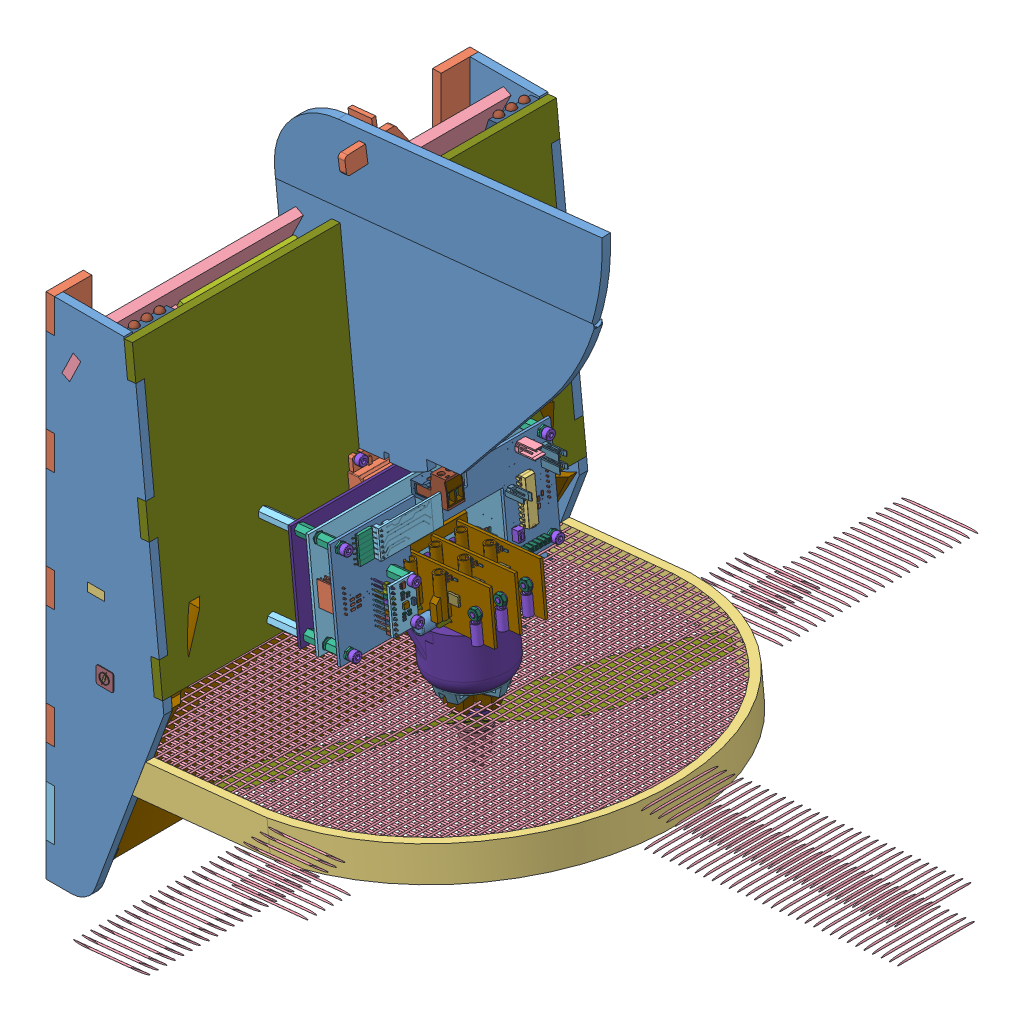
SolidWorks assembly AssTotale, configuration Défaut. Lengths in mm. (continued)
Components (placement in the parent): (continued)
- AssStructSimu-1: AssStructSimu [Défaut] at (-75.9431 -10.8604 24.5323) size (253.25 324.59 251.6) (continued)
  - AssCarte-1: AssCarte [Défaut] at (-42.8534 32.2132 302.028) x (-0.101852 0.9948 0) z (0.9948 0.101852 0) size (67.15 130.57 98.45) (continued)
    - carte_onduleur_v4-1: carte_onduleur_v4 [Défaut] at (-25.7639 0.8332 112.9379) size (66.52 130.57 82.34) (continued)
      - CARTE_CMD-1: CARTE_CMD [Défaut] at (25 57.2 0.803) size (60.1 130 26.71) (continued)
        - Open CASCADE STEP translator 6.8 1.20.1-1: Open CASCADE STEP translator 6.8 1.20.1 [Défaut] at origin size (60.1 130 26.71) (continued)
          - Body_1_4-1: Body_1_4 [Défaut] at (-55 5 12) size (60.1 130 26.71) (continued)
            - 175-1: 175 [Défaut] at (10 -21.7 0.803) x (0 -1 0) z (0 0 1) size (15 25.4 12.78) (continued)
              - =_[0_1_1_72]-1: =_[0_1_1_72] [Défaut] at origin size (15 25.4 12.78) (continued)
                - 173-1: 173 [Défaut] at (-1.4 -1 12) x (-1 0 0) z (0 1 0) size (15 12.78 25.4) (continued)
                  - RESC-0603_5-3: RESC-0603_5 [Défaut] at (-6.85 0 17.55) x (1 0 0) z (0 1 0) size (1.7 0.9 0.55) (continued)
                    - 152-1: 152 [Défaut] at origin (continued)
                      - =_[0_1_1_112]-1: =_[0_1_1_112] [Défaut] at origin
                      - =_[0_1_1_113]-1: =_[0_1_1_113] [Défaut] at origin
                      - =_[0_1_1_114]-1: =_[0_1_1_114] [Défaut] at origin
                      - =_[0_1_1_115]-1: =_[0_1_1_115] [Défaut] at origin
                  - RESC-0603_5-4: RESC-0603_5 [Défaut] at (-6.85 0 16.05) x (1 0 0) z (0 1 0) size (1.7 0.9 0.55)
                    - 143-1: 143 [Défaut] at origin size (1.7 0.9 0.55)
                      - =_[0_1_1_103]-1: =_[0_1_1_103] [Défaut] at origin size (0.4 0.9 0.53)
                      - =_[0_1_1_105]-1: =_[0_1_1_105] [Défaut] at origin size (0.4 0.9 0.53)
                      - =_[0_1_1_106]-1: =_[0_1_1_106] [Défaut] at origin size (1.64 0.9 0.52)
                    - 152-1: 152 [Défaut] at origin
                      - =_[0_1_1_107]-1: =_[0_1_1_107] [Défaut] at origin
                      - =_[0_1_1_109]-1: =_[0_1_1_109] [Défaut] at origin
                      - =_[0_1_1_110]-1: =_[0_1_1_110] [Défaut] at origin
                      - =_[0_1_1_111]-1: =_[0_1_1_111] [Défaut] at origin
                      - =_[0_1_1_112]-1: =_[0_1_1_112] [Défaut] at origin
                      - =_[0_1_1_113]-1: =_[0_1_1_113] [Défaut] at origin
                      - =_[0_1_1_114]-1: =_[0_1_1_114] [Défaut] at origin
                      - =_[0_1_1_115]-1: =_[0_1_1_115] [Défaut] at origin
                  - RESC-0603_5-5: RESC-0603_5 [Défaut] at (-6.85 0 5.95) x (1 0 0) z (0 1 0) size (1.7 0.9 0.55)
                    - 143-1: 143 [Défaut] at origin size (1.7 0.9 0.55)
                      - =_[0_1_1_103]-1: =_[0_1_1_103] [Défaut] at origin size (0.4 0.9 0.53)
                      - =_[0_1_1_105]-1: =_[0_1_1_105] [Défaut] at origin size (0.4 0.9 0.53)
                      - =_[0_1_1_106]-1: =_[0_1_1_106] [Défaut] at origin size (1.64 0.9 0.52)
                    - 152-1: 152 [Défaut] at origin
                      - =_[0_1_1_107]-1: =_[0_1_1_107] [Défaut] at origin
                      - =_[0_1_1_109]-1: =_[0_1_1_109] [Défaut] at origin
                      - =_[0_1_1_110]-1: =_[0_1_1_110] [Défaut] at origin
                      - =_[0_1_1_111]-1: =_[0_1_1_111] [Défaut] at origin
                      - =_[0_1_1_112]-1: =_[0_1_1_112] [Défaut] at origin
                      - =_[0_1_1_113]-1: =_[0_1_1_113] [Défaut] at origin
                      - =_[0_1_1_114]-1: =_[0_1_1_114] [Défaut] at origin
                      - =_[0_1_1_115]-1: =_[0_1_1_115] [Défaut] at origin
                  - CAPC-0603-T0.9-BN_5-1: CAPC-0603-T0.9-BN_5 [Défaut] at (-9.85 0 8.95) x (1 0 0) z (0 1 0) size (1.7 0.9 0.9)
                    - =_[0_1_1_117]-1: =_[0_1_1_117] [Défaut] at origin size (1.7 0.9 0.9)
                    - 167-1: 167 [Défaut] at origin
                      - =_[0_1_1_118]-1: =_[0_1_1_118] [Défaut] at origin
                      - =_[0_1_1_120]-1: =_[0_1_1_120] [Défaut] at origin
                      - =_[0_1_1_121]-1: =_[0_1_1_121] [Défaut] at origin
                      - =_[0_1_1_122]-1: =_[0_1_1_122] [Défaut] at origin
                      - =_[0_1_1_123]-1: =_[0_1_1_123] [Défaut] at origin
                      - =_[0_1_1_124]-1: =_[0_1_1_124] [Défaut] at origin
                      - =_[0_1_1_125]-1: =_[0_1_1_125] [Défaut] at origin
                      - =_[0_1_1_126]-1: =_[0_1_1_126] [Défaut] at origin
                  - CAPC-0603-T0.9-BN_5-2: CAPC-0603-T0.9-BN_5 [Défaut] at (-6.85 0 8.95) x (1 0 0) z (0 1 0) size (1.7 0.9 0.9)
                    - =_[0_1_1_117]-1: =_[0_1_1_117] [Défaut] at origin size (1.7 0.9 0.9)
                    - 167-1: 167 [Défaut] at origin
                      - =_[0_1_1_118]-1: =_[0_1_1_118] [Défaut] at origin
                      - =_[0_1_1_120]-1: =_[0_1_1_120] [Défaut] at origin
                      - =_[0_1_1_121]-1: =_[0_1_1_121] [Défaut] at origin
                      - =_[0_1_1_122]-1: =_[0_1_1_122] [Défaut] at origin
                      - =_[0_1_1_123]-1: =_[0_1_1_123] [Défaut] at origin
                      - =_[0_1_1_124]-1: =_[0_1_1_124] [Défaut] at origin
                      - =_[0_1_1_125]-1: =_[0_1_1_125] [Défaut] at origin
                      - =_[0_1_1_126]-1: =_[0_1_1_126] [Défaut] at origin
                  - CAPC-0603-T0.9-BN_5-3: CAPC-0603-T0.9-BN_5 [Défaut] at (-6.85 0 19.05) x (1 0 0) z (0 1 0) size (1.7 0.9 0.9)
                    - =_[0_1_1_117]-1: =_[0_1_1_117] [Défaut] at origin size (1.7 0.9 0.9)
                    - 167-1: 167 [Défaut] at origin
                      - =_[0_1_1_118]-1: =_[0_1_1_118] [Défaut] at origin
                      - =_[0_1_1_120]-1: =_[0_1_1_120] [Défaut] at origin
                      - =_[0_1_1_121]-1: =_[0_1_1_121] [Défaut] at origin
                      - =_[0_1_1_122]-1: =_[0_1_1_122] [Défaut] at origin
                      - =_[0_1_1_123]-1: =_[0_1_1_123] [Défaut] at origin
                      - =_[0_1_1_124]-1: =_[0_1_1_124] [Défaut] at origin
                      - =_[0_1_1_125]-1: =_[0_1_1_125] [Défaut] at origin
                      - =_[0_1_1_126]-1: =_[0_1_1_126] [Défaut] at origin
                  - CAPC-0603-T0.9-BN_5-4: CAPC-0603-T0.9-BN_5 [Défaut] at (-9.85 0 7.45) x (1 0 0) z (0 1 0) size (1.7 0.9 0.9)
                    - =_[0_1_1_117]-1: =_[0_1_1_117] [Défaut] at origin size (1.7 0.9 0.9)
                    - 167-1: 167 [Défaut] at origin
                      - =_[0_1_1_118]-1: =_[0_1_1_118] [Défaut] at origin
                      - =_[0_1_1_120]-1: =_[0_1_1_120] [Défaut] at origin
                      - =_[0_1_1_121]-1: =_[0_1_1_121] [Défaut] at origin
                      - =_[0_1_1_122]-1: =_[0_1_1_122] [Défaut] at origin
                      - =_[0_1_1_123]-1: =_[0_1_1_123] [Défaut] at origin
                      - =_[0_1_1_124]-1: =_[0_1_1_124] [Défaut] at origin
                      - =_[0_1_1_125]-1: =_[0_1_1_125] [Défaut] at origin
                      - =_[0_1_1_126]-1: =_[0_1_1_126] [Défaut] at origin
                  - CAPC-0603-T0.9-BN_5-5: CAPC-0603-T0.9-BN_5 [Défaut] at (-9.85 0 17.55) x (1 0 0) z (0 1 0) size (1.7 0.9 0.9)
                    - =_[0_1_1_117]-1: =_[0_1_1_117] [Défaut] at origin size (1.7 0.9 0.9)
                    - 167-1: 167 [Défaut] at origin
                      - =_[0_1_1_118]-1: =_[0_1_1_118] [Défaut] at origin
                      - =_[0_1_1_120]-1: =_[0_1_1_120] [Défaut] at origin
                      - =_[0_1_1_121]-1: =_[0_1_1_121] [Défaut] at origin
                      - =_[0_1_1_122]-1: =_[0_1_1_122] [Défaut] at origin
                      - =_[0_1_1_123]-1: =_[0_1_1_123] [Défaut] at origin
                      - =_[0_1_1_124]-1: =_[0_1_1_124] [Défaut] at origin
                      - =_[0_1_1_125]-1: =_[0_1_1_125] [Défaut] at origin
                      - =_[0_1_1_126]-1: =_[0_1_1_126] [Défaut] at origin
            - 177-1: 177 [Défaut] at (52.1 -16.5 -0.803) x (1 0 0) z (0 0 -1) size (2.34 1.04 0.5)
              - =_[0_1_1_30]-1: =_[0_1_1_30] [Défaut] at origin size (2.34 1.04 0.5)
                - 32_2-1: 32_2 [Défaut] at origin size (2.29 1.04 0.43)
                - 33_2-1: 33_2 [Défaut] at (0.3048 0 0) x (-1 0 0) z (0 0 1) size (0.51 1.02 0.5)
                - 34-1: 34 [Défaut] at origin size (0.51 1.02 0.5)
            - 179-1: 179 [Défaut] at (22.5336 -121.5 -0.803) x (-1 0 0) z (0 0 -1) size (2.34 1.04 0.5)
              - =_[0_1_1_30]-1: =_[0_1_1_30] [Défaut] at origin size (2.34 1.04 0.5)
                - 32_2-1: 32_2 [Défaut] at origin size (2.29 1.04 0.43)
                - 33_2-1: 33_2 [Défaut] at (0.3048 0 0) x (-1 0 0) z (0 0 1) size (0.51 1.02 0.5)
                - 34-1: 34 [Défaut] at origin size (0.51 1.02 0.5)
            - 181-1: 181 [Défaut] at (48.6 -127 -0.803) x (-1 0 0) z (0 0 -1) size (2.34 1.04 0.5)
              - =_[0_1_1_30]-1: =_[0_1_1_30] [Défaut] at origin size (2.34 1.04 0.5)
                - 32_2-1: 32_2 [Défaut] at origin size (2.29 1.04 0.43)
                - 33_2-1: 33_2 [Défaut] at (0.3048 0 0) x (-1 0 0) z (0 0 1) size (0.51 1.02 0.5)
                - 34-1: 34 [Défaut] at origin size (0.51 1.02 0.5)
            - 183-1: 183 [Défaut] at (26.0189 -121.5 0.803) size (2.34 1.04 0.5)
              - =_[0_1_1_30]-1: =_[0_1_1_30] [Défaut] at origin size (2.34 1.04 0.5)
                - 32_2-1: 32_2 [Défaut] at origin size (2.29 1.04 0.43)
                - 33_2-1: 33_2 [Défaut] at (0.3048 0 0) x (-1 0 0) z (0 0 1) size (0.51 1.02 0.5)
                - 34-1: 34 [Défaut] at origin size (0.51 1.02 0.5)
            - 185-1: 185 [Défaut] at (30.3664 -19 -0.803) x (1 0 0) z (0 0 -1) size (2.34 1.04 0.5)
              - =_[0_1_1_30]-1: =_[0_1_1_30] [Défaut] at origin size (2.34 1.04 0.5)
                - 32_2-1: 32_2 [Défaut] at origin size (2.29 1.04 0.43)
                - 33_2-1: 33_2 [Défaut] at (0.3048 0 0) x (-1 0 0) z (0 0 1) size (0.51 1.02 0.5)
                - 34-1: 34 [Défaut] at origin size (0.51 1.02 0.5)
            - 187-1: 187 [Défaut] at (51.7 -114.3 -0.803) x (0 1 0) z (0 0 -1) size (2.34 1.04 0.5)
              - =_[0_1_1_30]-1: =_[0_1_1_30] [Défaut] at origin size (2.34 1.04 0.5)
                - 32_2-1: 32_2 [Défaut] at origin size (2.29 1.04 0.43)
                - 33_2-1: 33_2 [Défaut] at (0.3048 0 0) x (-1 0 0) z (0 0 1) size (0.51 1.02 0.5)
                - 34-1: 34 [Défaut] at origin size (0.51 1.02 0.5)
            - 189-1: 189 [Défaut] at (50 -114.3 -0.803) x (0 1 0) z (0 0 -1) size (2.34 1.04 0.5)
              - =_[0_1_1_30]-1: =_[0_1_1_30] [Défaut] at origin size (2.34 1.04 0.5)
                - 32_2-1: 32_2 [Défaut] at origin size (2.29 1.04 0.43)
                - 33_2-1: 33_2 [Défaut] at (0.3048 0 0) x (-1 0 0) z (0 0 1) size (0.51 1.02 0.5)
                - 34-1: 34 [Défaut] at origin size (0.51 1.02 0.5)
            - 192-1: 192 [Défaut] at (37.94 -103.3308 0.803) x (-1 0 0) z (0 0 1) size (5.08 5 14.3)
              - =_[0_1_1_135]-1: =_[0_1_1_135] [Défaut] at origin size (5.08 5 14.3)
                - 190-1: 190 [Défaut] at (1.2 0 11) size (5.08 5 14.3)
            - 194-1: 194 [Défaut] at (32.7796 -102.6 -0.803) x (-1 0 0) z (0 0 -1) size (2.54 1.98 0.64)
              - =_[0_1_1_46]-1: =_[0_1_1_46] [Défaut] at origin size (2.54 1.98 0.64)
                - 52-1: 52 [Défaut] at origin size (2.54 1.14 0.58)
                - 53-1: 53 [Défaut] x (0 -1 0) z (0 0 1) size (0.43 0.51 0.38)
                - 54-1: 54 [Défaut] at (1.8796 1.8796 0) x (0 -1 0) z (0 0 1) size (0.43 0.51 0.38)
                - 55-1: 55 [Défaut] at (-0.9652 -2.8448 0) x (0 1 0) z (0 0 1) size (0.41 0.51 0.38)
            - 196-1: 196 [Défaut] at (40.243 -104.3176 -0.803) x (0 1 0) z (0 0 -1) size (2.34 1.04 0.5)
              - =_[0_1_1_30]-1: =_[0_1_1_30] [Défaut] at origin size (2.34 1.04 0.5)
                - 32_2-1: 32_2 [Défaut] at origin size (2.29 1.04 0.43)
                - 33_2-1: 33_2 [Défaut] at (0.3048 0 0) x (-1 0 0) z (0 0 1) size (0.51 1.02 0.5)
                - 34-1: 34 [Défaut] at origin size (0.51 1.02 0.5)
            - 198-1: 198 [Défaut] at (42 -104.3176 -0.803) x (0 1 0) z (0 0 -1) size (2.34 1.04 0.5)
              - =_[0_1_1_30]-1: =_[0_1_1_30] [Défaut] at origin size (2.34 1.04 0.5)
                - 32_2-1: 32_2 [Défaut] at origin size (2.29 1.04 0.43)
                - 33_2-1: 33_2 [Défaut] at (0.3048 0 0) x (-1 0 0) z (0 0 1) size (0.51 1.02 0.5)
                - 34-1: 34 [Défaut] at origin size (0.51 1.02 0.5)
            - 200-1: 200 [Défaut] at (30.1 -112.9336 -0.803) x (0 1 0) z (0 0 -1) size (2.34 1.04 0.5)
              - =_[0_1_1_30]-1: =_[0_1_1_30] [Défaut] at origin size (2.34 1.04 0.5)
                - 32_2-1: 32_2 [Défaut] at origin size (2.29 1.04 0.43)
                - 33_2-1: 33_2 [Défaut] at (0.3048 0 0) x (-1 0 0) z (0 0 1) size (0.51 1.02 0.5)
                - 34-1: 34 [Défaut] at origin size (0.51 1.02 0.5)
      - C2_1-1: C2_1 [Défaut] at (-20.6984 1.8 -0.803) x (1 0 0) z (0 0 -1) size (2.34 1.04 0.5)
        - Open CASCADE STEP translator 6.8 1.6.1-1: Open CASCADE STEP translator 6.8 1.6.1 [Défaut] at origin size (2.34 1.04 0.5)
          - Body_1-1: Body_1 [Défaut] at origin size (2.29 1.04 0.43)
          - Pin_1-1: Pin_1 [Défaut] at (0.3048 0 0) x (-1 0 0) z (0 0 1) size (0.51 1.02 0.5)
          - Pin_2-1: Pin_2 [Défaut] at origin size (0.51 1.02 0.5)
      - C2_2-1: C2_2 [Défaut] at (-24.2 1.8 -0.803) x (1 0 0) z (0 0 -1) size (2.34 1.04 0.5)
        - Open CASCADE STEP translator 6.8 1.6.1-1: Open CASCADE STEP translator 6.8 1.6.1 [Défaut] at origin size (2.34 1.04 0.5)
          - Body_1-1: Body_1 [Défaut] at origin size (2.29 1.04 0.43)
          - Pin_1-1: Pin_1 [Défaut] at (0.3048 0 0) x (-1 0 0) z (0 0 1) size (0.51 1.02 0.5)
          - Pin_2-1: Pin_2 [Défaut] at origin size (0.51 1.02 0.5)
      - C3_1-1: C3_1 [Défaut] at (-20.9176 -12.8 -0.803) x (1 0 0) z (0 0 -1) size (2.34 1.04 0.5)
        - Open CASCADE STEP translator 6.8 1.6.1-1: Open CASCADE STEP translator 6.8 1.6.1 [Défaut] at origin size (2.34 1.04 0.5)
          - Body_1-1: Body_1 [Défaut] at origin size (2.29 1.04 0.43)
          - Pin_1-1: Pin_1 [Défaut] at (0.3048 0 0) x (-1 0 0) z (0 0 1) size (0.51 1.02 0.5)
          - Pin_2-1: Pin_2 [Défaut] at origin size (0.51 1.02 0.5)
      - C3_2-1: C3_2 [Défaut] at (-24.4 -12.8 -0.803) x (1 0 0) z (0 0 -1) size (2.34 1.04 0.5)
        - Open CASCADE STEP translator 6.8 1.6.1-1: Open CASCADE STEP translator 6.8 1.6.1 [Défaut] at origin size (2.34 1.04 0.5)
          - Body_1-1: Body_1 [Défaut] at origin size (2.29 1.04 0.43)
          - Pin_1-1: Pin_1 [Défaut] at (0.3048 0 0) x (-1 0 0) z (0 0 1) size (0.51 1.02 0.5)
          - Pin_2-1: Pin_2 [Défaut] at origin size (0.51 1.02 0.5)
      - D_CUR-1: D_CUR [Défaut] at (-12.4432 3.85 -0.803) x (0 -1 0) z (0 0 -1) size (2.7 5.2 1.11)
        - Open CASCADE STEP translator 6.8 1.25.1-1: Open CASCADE STEP translator 6.8 1.25.1 [Défaut] at origin size (2.7 5.2 1.11)
          - Body_1_5-1: Body_1_5 [Défaut] at (1.2 -4 0) x (0 1 0) z (0 0 1) size (5.2 2.7 1.11)
            - =_[0_1_1_3]_4-1: =_[0_1_1_3]_4 [Défaut] at origin size (0.39 0.64 0.01)
            - =_[0_1_1_4]_4-1: =_[0_1_1_4]_4 [Défaut] at origin size (0.6 1.9 0.2)
            - =_[0_1_1_5]_4-1: =_[0_1_1_5]_4 [Défaut] at origin size (0.21 0.08 0.01)
            - =_[0_1_1_6]_2-1: =_[0_1_1_6]_2 [Défaut] at origin size (0.6 1.9 0.2)
            - =_[0_1_1_7]_2-1: =_[0_1_1_7]_2 [Défaut] at origin size (0.46 0.68 0.01)
            - =_[0_1_1_8]_2-1: =_[0_1_1_8]_2 [Défaut] at origin size (0.38 0.66 0.01)
            - =_[0_1_1_9]-1: =_[0_1_1_9] [Défaut] at origin size (0.2 0.62 0.01)
            - =_[0_1_1_10]-1: =_[0_1_1_10] [Défaut] at origin size (4 2.7 1.1)
            - =_[0_1_1_11]-1: =_[0_1_1_11] [Défaut] at origin size (0.46 0.63 0.01)
            - =_[0_1_1_12]-1: =_[0_1_1_12] [Défaut] at origin size (0.56 0.68 0.01)
      - RC1_1-1: RC1_1 [Défaut] at (-20.7176 8.1 -0.803) x (1 0 0) z (0 0 -1) size (2.34 1.04 0.5)
        - Open CASCADE STEP translator 6.8 1.12.1-1: Open CASCADE STEP translator 6.8 1.12.1 [Défaut] at origin size (2.34 1.04 0.5)
          - Body_1_3-1: Body_1_3 [Défaut] at origin size (2.29 1.04 0.43)
          - Pin_1_2-1: Pin_1_2 [Défaut] at (0.3048 0 0) x (-1 0 0) z (0 0 1) size (0.51 1.02 0.5)
          - Pin_2_2-1: Pin_2_2 [Défaut] at origin size (0.51 1.02 0.5)
      - RC1_2-1: RC1_2 [Défaut] at (-22 8.1 -0.803) x (-1 0 0) z (0 0 -1) size (2.34 1.04 0.5)
        - Open CASCADE STEP translator 6.8 1.12.1-1: Open CASCADE STEP translator 6.8 1.12.1 [Défaut] at origin size (2.34 1.04 0.5)
          - Body_1_3-1: Body_1_3 [Défaut] at origin size (2.29 1.04 0.43)
          - Pin_1_2-1: Pin_1_2 [Défaut] at (0.3048 0 0) x (-1 0 0) z (0 0 1) size (0.51 1.02 0.5)
          - Pin_2_2-1: Pin_2_2 [Défaut] at origin size (0.51 1.02 0.5)
      - RC2_1-1: RC2_1 [Défaut] at (-20.716 0.243 -0.803) x (1 0 0) z (0 0 -1) size (2.34 1.04 0.5)
        - Open CASCADE STEP translator 6.8 1.12.1-1: Open CASCADE STEP translator 6.8 1.12.1 [Défaut] at origin size (2.34 1.04 0.5)
          - Body_1_3-1: Body_1_3 [Défaut] at origin size (2.29 1.04 0.43)
          - Pin_1_2-1: Pin_1_2 [Défaut] at (0.3048 0 0) x (-1 0 0) z (0 0 1) size (0.51 1.02 0.5)
          - Pin_2_2-1: Pin_2_2 [Défaut] at origin size (0.51 1.02 0.5)
      - RC2_2-1: RC2_2 [Défaut] at (-22 0.18 -0.803) x (-1 0 0) z (0 0 -1) size (2.34 1.04 0.5)
        - Open CASCADE STEP translator 6.8 1.12.1-1: Open CASCADE STEP translator 6.8 1.12.1 [Défaut] at origin size (2.34 1.04 0.5)
          - Body_1_3-1: Body_1_3 [Défaut] at origin size (2.29 1.04 0.43)
          - Pin_1_2-1: Pin_1_2 [Défaut] at (0.3048 0 0) x (-1 0 0) z (0 0 1) size (0.51 1.02 0.5)
          - Pin_2_2-1: Pin_2_2 [Défaut] at origin size (0.51 1.02 0.5)
      - RC3_1-1: RC3_1 [Défaut] at (-20.9336 -14.5 -0.803) x (1 0 0) z (0 0 -1) size (2.34 1.04 0.5)
        - Open CASCADE STEP translator 6.8 1.12.1-1: Open CASCADE STEP translator 6.8 1.12.1 [Défaut] at origin size (2.34 1.04 0.5)
          - Body_1_3-1: Body_1_3 [Défaut] at origin size (2.29 1.04 0.43)
          - Pin_1_2-1: Pin_1_2 [Défaut] at (0.3048 0 0) x (-1 0 0) z (0 0 1) size (0.51 1.02 0.5)
          - Pin_2_2-1: Pin_2_2 [Défaut] at origin size (0.51 1.02 0.5)
      - RC3_2-1: RC3_2 [Défaut] at (-22.3 -14.5 -0.803) x (-1 0 0) z (0 0 -1) size (2.34 1.04 0.5)
        - Open CASCADE STEP translator 6.8 1.12.1-1: Open CASCADE STEP translator 6.8 1.12.1 [Défaut] at origin size (2.34 1.04 0.5)
          - Body_1_3-1: Body_1_3 [Défaut] at origin size (2.29 1.04 0.43)
          - Pin_1_2-1: Pin_1_2 [Défaut] at (0.3048 0 0) x (-1 0 0) z (0 0 1) size (0.51 1.02 0.5)
          - Pin_2_2-1: Pin_2_2 [Défaut] at origin size (0.51 1.02 0.5)
      - U_MES_CUR-1: U_MES_CUR [Défaut] at (-11.5 6.7816 0.803) size (2.54 2.41 0.76)
        - Open CASCADE STEP translator 6.8 1.32.1-1: Open CASCADE STEP translator 6.8 1.32.1 [Défaut] at origin size (2.54 2.41 0.76)
          - Body_1_5-1: Body_1_5 [Défaut] at origin size (2.54 1.27 0.71)
          - Pin_1_3-1: Pin_1_3 [Défaut] at (-2.1082 0.2286 0) x (0 -1 0) z (0 0 1) size (1.14 0.25 0.47)
          - Pin_2_3-1: Pin_2_3 [Défaut] at (-0.2032 2.1336 0) x (0 -1 0) z (0 0 1) size (1.14 0.25 0.47)
      - COMP1-1: COMP1 [Défaut] at (-16.3 -36.2 0.803) x (-1 0 0) z (0 0 1) size (2.03 1.88 0.51)
        - Open CASCADE STEP translator 6.8 1.33.1-1: Open CASCADE STEP translator 6.8 1.33.1 [Défaut] at origin size (2.03 1.88 0.51)
          - Body_1_6-1: Body_1_6 [Défaut] at origin size (2.03 1.02 0.46)
          - Pin_1_4-1: Pin_1_4 [Défaut] x (0 1 0) z (0 0 1) size (0.45 0.25 0.32)
          - Pin_2_4-1: Pin_2_4 [Défaut] at (0.65 -0.65 0) x (0 1 0) z (0 0 1) size (0.45 0.25 0.32)
          - Pin_3-1: Pin_3 [Défaut] at (1.3 -1.3 0) x (0 1 0) z (0 0 1) size (0.45 0.25 0.32)
          - Pin_4-1: Pin_4 [Défaut] at (-0.5 3.1 0) x (0 -1 0) z (0 0 1) size (0.41 0.25 0.32)
          - Pin_5-1: Pin_5 [Défaut] at (-1.8 1.8 0) x (0 -1 0) z (0 0 1) size (0.41 0.25 0.32)
      - COMP2-1: COMP2 [Défaut] at (-14.3 -9.6 0.803) x (-1 0 0) z (0 0 1) size (2.03 1.88 0.51)
        - Open CASCADE STEP translator 6.8 1.33.1-1: Open CASCADE STEP translator 6.8 1.33.1 [Défaut] at origin size (2.03 1.88 0.51)
          - Body_1_6-1: Body_1_6 [Défaut] at origin size (2.03 1.02 0.46)
          - Pin_1_4-1: Pin_1_4 [Défaut] x (0 1 0) z (0 0 1) size (0.45 0.25 0.32)
          - Pin_2_4-1: Pin_2_4 [Défaut] at (0.65 -0.65 0) x (0 1 0) z (0 0 1) size (0.45 0.25 0.32)
          - Pin_3-1: Pin_3 [Défaut] at (1.3 -1.3 0) x (0 1 0) z (0 0 1) size (0.45 0.25 0.32)
          - Pin_4-1: Pin_4 [Défaut] at (-0.5 3.1 0) x (0 -1 0) z (0 0 1) size (0.41 0.25 0.32)
          - Pin_5-1: Pin_5 [Défaut] at (-1.8 1.8 0) x (0 -1 0) z (0 0 1) size (0.41 0.25 0.32)
      - COMP3-1: COMP3 [Défaut] at (-15.9 -23.2 0.803) x (-1 0 0) z (0 0 1) size (2.03 1.88 0.51)
        - Open CASCADE STEP translator 6.8 1.33.1-1: Open CASCADE STEP translator 6.8 1.33.1 [Défaut] at origin size (2.03 1.88 0.51)
          - Body_1_6-1: Body_1_6 [Défaut] at origin size (2.03 1.02 0.46)
          - Pin_1_4-1: Pin_1_4 [Défaut] x (0 1 0) z (0 0 1) size (0.45 0.25 0.32)
          - Pin_2_4-1: Pin_2_4 [Défaut] at (0.65 -0.65 0) x (0 1 0) z (0 0 1) size (0.45 0.25 0.32)
          - Pin_3-1: Pin_3 [Défaut] at (1.3 -1.3 0) x (0 1 0) z (0 0 1) size (0.45 0.25 0.32)
          - Pin_4-1: Pin_4 [Défaut] at (-0.5 3.1 0) x (0 -1 0) z (0 0 1) size (0.41 0.25 0.32)
          - Pin_5-1: Pin_5 [Défaut] at (-1.8 1.8 0) x (0 -1 0) z (0 0 1) size (0.41 0.25 0.32)
      - CP1-1: CP1 [Défaut] at (-18.9 -38.2 0.803) x (0 1 0) z (0 0 1) size (2.34 1.04 0.5)
        - Open CASCADE STEP translator 6.8 1.6.1-1: Open CASCADE STEP translator 6.8 1.6.1 [Défaut] at origin size (2.34 1.04 0.5)
          - Body_1-1: Body_1 [Défaut] at origin size (2.29 1.04 0.43)
          - Pin_1-1: Pin_1 [Défaut] at (0.3048 0 0) x (-1 0 0) z (0 0 1) size (0.51 1.02 0.5)
          - Pin_2-1: Pin_2 [Défaut] at origin size (0.51 1.02 0.5)
      - CP2-1: CP2 [Défaut] at (-16.9 -11.6 0.803) x (0 1 0) z (0 0 1) size (2.34 1.04 0.5)
        - Open CASCADE STEP translator 6.8 1.6.1-1: Open CASCADE STEP translator 6.8 1.6.1 [Défaut] at origin size (2.34 1.04 0.5)
          - Body_1-1: Body_1 [Défaut] at origin size (2.29 1.04 0.43)
          - Pin_1-1: Pin_1 [Défaut] at (0.3048 0 0) x (-1 0 0) z (0 0 1) size (0.51 1.02 0.5)
          - Pin_2-1: Pin_2 [Défaut] at origin size (0.51 1.02 0.5)
      - CP3-1: CP3 [Défaut] at (-18.5 -25.2 0.803) x (0 1 0) z (0 0 1) size (2.34 1.04 0.5)
        - Open CASCADE STEP translator 6.8 1.6.1-1: Open CASCADE STEP translator 6.8 1.6.1 [Défaut] at origin size (2.34 1.04 0.5)
          - Body_1-1: Body_1 [Défaut] at origin size (2.29 1.04 0.43)
          - Pin_1-1: Pin_1 [Défaut] at (0.3048 0 0) x (-1 0 0) z (0 0 1) size (0.51 1.02 0.5)
          - Pin_2-1: Pin_2 [Défaut] at origin size (0.51 1.02 0.5)
      - C_DEC_COM1-1: C_DEC_COM1 [Défaut] at (-15 -36 0.803) x (0 -1 0) z (0 0 1) size (2.34 1.04 0.5)
        - Open CASCADE STEP translator 6.8 1.6.1-1: Open CASCADE STEP translator 6.8 1.6.1 [Défaut] at origin size (2.34 1.04 0.5)
          - Body_1-1: Body_1 [Défaut] at origin size (2.29 1.04 0.43)
          - Pin_1-1: Pin_1 [Défaut] at (0.3048 0 0) x (-1 0 0) z (0 0 1) size (0.51 1.02 0.5)
          - Pin_2-1: Pin_2 [Défaut] at origin size (0.51 1.02 0.5)
      - C_DEC_COMP2-1: C_DEC_COMP2 [Défaut] at (-13 -9.3 0.803) x (0 -1 0) z (0 0 1) size (2.34 1.04 0.5)
        - Open CASCADE STEP translator 6.8 1.6.1-1: Open CASCADE STEP translator 6.8 1.6.1 [Défaut] at origin size (2.34 1.04 0.5)
          - Body_1-1: Body_1 [Défaut] at origin size (2.29 1.04 0.43)
          - Pin_1-1: Pin_1 [Défaut] at (0.3048 0 0) x (-1 0 0) z (0 0 1) size (0.51 1.02 0.5)
          - Pin_2-1: Pin_2 [Défaut] at origin size (0.51 1.02 0.5)
      - C_DEC_COMP3-1: C_DEC_COMP3 [Défaut] at (-14.6 -22.9 0.803) x (0 -1 0) z (0 0 1) size (2.34 1.04 0.5)
        - Open CASCADE STEP translator 6.8 1.6.1-1: Open CASCADE STEP translator 6.8 1.6.1 [Défaut] at origin size (2.34 1.04 0.5)
          - Body_1-1: Body_1 [Défaut] at origin size (2.29 1.04 0.43)
          - Pin_1-1: Pin_1 [Défaut] at (0.3048 0 0) x (-1 0 0) z (0 0 1) size (0.51 1.02 0.5)
          - Pin_2-1: Pin_2 [Défaut] at origin size (0.51 1.02 0.5)
      - D_VBAT-1: D_VBAT [Défaut] at (-1.2 46.4 0.803) x (0 -1 0) z (0 0 1) size (2.34 1.04 0.5)
        - Open CASCADE STEP translator 6.8 1.6.1-1: Open CASCADE STEP translator 6.8 1.6.1 [Défaut] at origin size (2.34 1.04 0.5)
          - Body_1-1: Body_1 [Défaut] at origin size (2.29 1.04 0.43)
          - Pin_1-1: Pin_1 [Défaut] at (0.3048 0 0) x (-1 0 0) z (0 0 1) size (0.51 1.02 0.5)
          - Pin_2-1: Pin_2 [Défaut] at origin size (0.51 1.02 0.5)
      - D_3V-1: D_3V [Défaut] at (1.3 46.3 0.803) x (0 -1 0) z (0 0 1) size (2.34 1.04 0.5)
        - Open CASCADE STEP translator 6.8 1.6.1-1: Open CASCADE STEP translator 6.8 1.6.1 [Défaut] at origin size (2.34 1.04 0.5)
          - Body_1-1: Body_1 [Défaut] at origin size (2.29 1.04 0.43)
          - Pin_1-1: Pin_1 [Défaut] at (0.3048 0 0) x (-1 0 0) z (0 0 1) size (0.51 1.02 0.5)
          - Pin_2-1: Pin_2 [Défaut] at origin size (0.51 1.02 0.5)
      - D_5V-1: D_5V [Défaut] at (-3.7 46.4 0.803) x (0 -1 0) z (0 0 1) size (2.34 1.04 0.5)
        - Open CASCADE STEP translator 6.8 1.6.1-1: Open CASCADE STEP translator 6.8 1.6.1 [Défaut] at origin size (2.34 1.04 0.5)
          - Body_1-1: Body_1 [Défaut] at origin size (2.29 1.04 0.43)
          - Pin_1-1: Pin_1 [Défaut] at (0.3048 0 0) x (-1 0 0) z (0 0 1) size (0.51 1.02 0.5)
          - Pin_2-1: Pin_2 [Défaut] at origin size (0.51 1.02 0.5)
      - R1_1-1: R1_1 [Défaut] at (-20.2 -36.1 0.803) x (-1 0 0) z (0 0 1) size (2.34 1.04 0.5)
        - Open CASCADE STEP translator 6.8 1.12.1-1: Open CASCADE STEP translator 6.8 1.12.1 [Défaut] at origin size (2.34 1.04 0.5)
          - Body_1_3-1: Body_1_3 [Défaut] at origin size (2.29 1.04 0.43)
          - Pin_1_2-1: Pin_1_2 [Défaut] at (0.3048 0 0) x (-1 0 0) z (0 0 1) size (0.51 1.02 0.5)
          - Pin_2_2-1: Pin_2_2 [Défaut] at origin size (0.51 1.02 0.5)
      - R1_2-1: R1_2 [Défaut] at (-15.5 -34.6 0.803) x (-1 0 0) z (0 0 1) size (2.34 1.04 0.5)
        - Open CASCADE STEP translator 6.8 1.12.1-1: Open CASCADE STEP translator 6.8 1.12.1 [Défaut] at origin size (2.34 1.04 0.5)
          - Body_1_3-1: Body_1_3 [Défaut] at origin size (2.29 1.04 0.43)
          - Pin_1_2-1: Pin_1_2 [Défaut] at (0.3048 0 0) x (-1 0 0) z (0 0 1) size (0.51 1.02 0.5)
          - Pin_2_2-1: Pin_2_2 [Défaut] at origin size (0.51 1.02 0.5)
      - R1_3-1: R1_3 [Défaut] at (-20.3 -39.9 0.803) x (-1 0 0) z (0 0 1) size (2.34 1.04 0.5)
        - Open CASCADE STEP translator 6.8 1.12.1-1: Open CASCADE STEP translator 6.8 1.12.1 [Défaut] at origin size (2.34 1.04 0.5)
          - Body_1_3-1: Body_1_3 [Défaut] at origin size (2.29 1.04 0.43)
          - Pin_1_2-1: Pin_1_2 [Défaut] at (0.3048 0 0) x (-1 0 0) z (0 0 1) size (0.51 1.02 0.5)
          - Pin_2_2-1: Pin_2_2 [Défaut] at origin size (0.51 1.02 0.5)
      - R1_4-1: R1_4 [Défaut] at (-20.3 -38.1 0.803) x (-1 0 0) z (0 0 1) size (2.34 1.04 0.5)
        - Open CASCADE STEP translator 6.8 1.12.1-1: Open CASCADE STEP translator 6.8 1.12.1 [Défaut] at origin size (2.34 1.04 0.5)
          - Body_1_3-1: Body_1_3 [Défaut] at origin size (2.29 1.04 0.43)
          - Pin_1_2-1: Pin_1_2 [Défaut] at (0.3048 0 0) x (-1 0 0) z (0 0 1) size (0.51 1.02 0.5)
          - Pin_2_2-1: Pin_2_2 [Défaut] at origin size (0.51 1.02 0.5)
      - R1_5-1: R1_5 [Défaut] at (-17.1336 -39.7 0.803) size (2.34 1.04 0.5)
        - Open CASCADE STEP translator 6.8 1.12.1-1: Open CASCADE STEP translator 6.8 1.12.1 [Défaut] at origin size (2.34 1.04 0.5)
          - Body_1_3-1: Body_1_3 [Défaut] at origin size (2.29 1.04 0.43)
          - Pin_1_2-1: Pin_1_2 [Défaut] at (0.3048 0 0) x (-1 0 0) z (0 0 1) size (0.51 1.02 0.5)
          - Pin_2_2-1: Pin_2_2 [Défaut] at origin size (0.51 1.02 0.5)
      - R2_1-1: R2_1 [Défaut] at (-18.5 -9.5 0.803) x (-1 0 0) z (0 0 1) size (2.34 1.04 0.5)
        - Open CASCADE STEP translator 6.8 1.12.1-1: Open CASCADE STEP translator 6.8 1.12.1 [Défaut] at origin size (2.34 1.04 0.5)
          - Body_1_3-1: Body_1_3 [Défaut] at origin size (2.29 1.04 0.43)
          - Pin_1_2-1: Pin_1_2 [Défaut] at (0.3048 0 0) x (-1 0 0) z (0 0 1) size (0.51 1.02 0.5)
          - Pin_2_2-1: Pin_2_2 [Défaut] at origin size (0.51 1.02 0.5)
      - R2_2-1: R2_2 [Défaut] at (-13.1 -8 0.803) x (-1 0 0) z (0 0 1) size (2.34 1.04 0.5)
        - Open CASCADE STEP translator 6.8 1.12.1-1: Open CASCADE STEP translator 6.8 1.12.1 [Défaut] at origin size (2.34 1.04 0.5)
          - Body_1_3-1: Body_1_3 [Défaut] at origin size (2.29 1.04 0.43)
          - Pin_1_2-1: Pin_1_2 [Défaut] at (0.3048 0 0) x (-1 0 0) z (0 0 1) size (0.51 1.02 0.5)
          - Pin_2_2-1: Pin_2_2 [Défaut] at origin size (0.51 1.02 0.5)
      - R2_3-1: R2_3 [Défaut] at (-18.5 -11.2 0.803) x (-1 0 0) z (0 0 1) size (2.34 1.04 0.5)
        - Open CASCADE STEP translator 6.8 1.12.1-1: Open CASCADE STEP translator 6.8 1.12.1 [Défaut] at origin size (2.34 1.04 0.5)
          - Body_1_3-1: Body_1_3 [Défaut] at origin size (2.29 1.04 0.43)
          - Pin_1_2-1: Pin_1_2 [Défaut] at (0.3048 0 0) x (-1 0 0) z (0 0 1) size (0.51 1.02 0.5)
          - Pin_2_2-1: Pin_2_2 [Défaut] at origin size (0.51 1.02 0.5)
      - R2_4-1: R2_4 [Défaut] at (-18.5 -12.8 0.803) x (-1 0 0) z (0 0 1) size (2.34 1.04 0.5)
        - Open CASCADE STEP translator 6.8 1.12.1-1: Open CASCADE STEP translator 6.8 1.12.1 [Défaut] at origin size (2.34 1.04 0.5)
          - Body_1_3-1: Body_1_3 [Défaut] at origin size (2.29 1.04 0.43)
          - Pin_1_2-1: Pin_1_2 [Défaut] at (0.3048 0 0) x (-1 0 0) z (0 0 1) size (0.51 1.02 0.5)
          - Pin_2_2-1: Pin_2_2 [Défaut] at origin size (0.51 1.02 0.5)
      - R2_5-1: R2_5 [Défaut] at (-15.1336 -13 0.803) size (2.34 1.04 0.5)
        - Open CASCADE STEP translator 6.8 1.12.1-1: Open CASCADE STEP translator 6.8 1.12.1 [Défaut] at origin size (2.34 1.04 0.5)
          - Body_1_3-1: Body_1_3 [Défaut] at origin size (2.29 1.04 0.43)
          - Pin_1_2-1: Pin_1_2 [Défaut] at (0.3048 0 0) x (-1 0 0) z (0 0 1) size (0.51 1.02 0.5)
          - Pin_2_2-1: Pin_2_2 [Défaut] at origin size (0.51 1.02 0.5)
      - R3_1-1: R3_1 [Défaut] at (-19.9 -23.1 0.803) x (-1 0 0) z (0 0 1) size (2.34 1.04 0.5)
        - Open CASCADE STEP translator 6.8 1.12.1-1: Open CASCADE STEP translator 6.8 1.12.1 [Défaut] at origin size (2.34 1.04 0.5)
          - Body_1_3-1: Body_1_3 [Défaut] at origin size (2.29 1.04 0.43)
          - Pin_1_2-1: Pin_1_2 [Défaut] at (0.3048 0 0) x (-1 0 0) z (0 0 1) size (0.51 1.02 0.5)
          - Pin_2_2-1: Pin_2_2 [Défaut] at origin size (0.51 1.02 0.5)
      - R3_2-1: R3_2 [Défaut] at (-14.7 -21.6 0.803) x (-1 0 0) z (0 0 1) size (2.34 1.04 0.5)
        - Open CASCADE STEP translator 6.8 1.12.1-1: Open CASCADE STEP translator 6.8 1.12.1 [Défaut] at origin size (2.34 1.04 0.5)
          - Body_1_3-1: Body_1_3 [Défaut] at origin size (2.29 1.04 0.43)
          - Pin_1_2-1: Pin_1_2 [Défaut] at (0.3048 0 0) x (-1 0 0) z (0 0 1) size (0.51 1.02 0.5)
          - Pin_2_2-1: Pin_2_2 [Défaut] at origin size (0.51 1.02 0.5)
      - R3_3-1: R3_3 [Défaut] at (-19.9 -24.8 0.803) x (-1 0 0) z (0 0 1) size (2.34 1.04 0.5)
        - Open CASCADE STEP translator 6.8 1.12.1-1: Open CASCADE STEP translator 6.8 1.12.1 [Défaut] at origin size (2.34 1.04 0.5)
          - Body_1_3-1: Body_1_3 [Défaut] at origin size (2.29 1.04 0.43)
          - Pin_1_2-1: Pin_1_2 [Défaut] at (0.3048 0 0) x (-1 0 0) z (0 0 1) size (0.51 1.02 0.5)
          - Pin_2_2-1: Pin_2_2 [Défaut] at origin size (0.51 1.02 0.5)
      - R3_4-1: R3_4 [Défaut] at (-19.9 -26.4 0.803) x (-1 0 0) z (0 0 1) size (2.34 1.04 0.5)
        - Open CASCADE STEP translator 6.8 1.12.1-1: Open CASCADE STEP translator 6.8 1.12.1 [Défaut] at origin size (2.34 1.04 0.5)
          - Body_1_3-1: Body_1_3 [Défaut] at origin size (2.29 1.04 0.43)
          - Pin_1_2-1: Pin_1_2 [Défaut] at (0.3048 0 0) x (-1 0 0) z (0 0 1) size (0.51 1.02 0.5)
          - Pin_2_2-1: Pin_2_2 [Défaut] at origin size (0.51 1.02 0.5)
      - R3_5-1: R3_5 [Défaut] at (-16.7336 -26.5 0.803) size (2.34 1.04 0.5)
        - Open CASCADE STEP translator 6.8 1.12.1-1: Open CASCADE STEP translator 6.8 1.12.1 [Défaut] at origin size (2.34 1.04 0.5)
          - Body_1_3-1: Body_1_3 [Défaut] at origin size (2.29 1.04 0.43)
          - Pin_1_2-1: Pin_1_2 [Défaut] at (0.3048 0 0) x (-1 0 0) z (0 0 1) size (0.51 1.02 0.5)
          - Pin_2_2-1: Pin_2_2 [Défaut] at origin size (0.51 1.02 0.5)
      - R_LED_3V3-1: R_LED_3V3 [Défaut] at (1.3 47.9 0.803) x (0 1 0) z (0 0 1) size (2.34 1.04 0.5)
        - Open CASCADE STEP translator 6.8 1.12.1-1: Open CASCADE STEP translator 6.8 1.12.1 [Défaut] at origin size (2.34 1.04 0.5)
          - Body_1_3-1: Body_1_3 [Défaut] at origin size (2.29 1.04 0.43)
          - Pin_1_2-1: Pin_1_2 [Défaut] at (0.3048 0 0) x (-1 0 0) z (0 0 1) size (0.51 1.02 0.5)
          - Pin_2_2-1: Pin_2_2 [Défaut] at origin size (0.51 1.02 0.5)
      - R_LED_5V-1: R_LED_5V [Défaut] at (-3.7 47.7 0.803) x (0 1 0) z (0 0 1) size (2.34 1.04 0.5)
        - Open CASCADE STEP translator 6.8 1.12.1-1: Open CASCADE STEP translator 6.8 1.12.1 [Défaut] at origin size (2.34 1.04 0.5)
          - Body_1_3-1: Body_1_3 [Défaut] at origin size (2.29 1.04 0.43)
          - Pin_1_2-1: Pin_1_2 [Défaut] at (0.3048 0 0) x (-1 0 0) z (0 0 1) size (0.51 1.02 0.5)
          - Pin_2_2-1: Pin_2_2 [Défaut] at origin size (0.51 1.02 0.5)
      - R_LED_VBAT-1: R_LED_VBAT [Défaut] at (-1.2 47.9 0.803) x (0 1 0) z (0 0 1) size (2.34 1.04 0.5)
        - Open CASCADE STEP translator 6.8 1.12.1-1: Open CASCADE STEP translator 6.8 1.12.1 [Défaut] at origin size (2.34 1.04 0.5)
          - Body_1_3-1: Body_1_3 [Défaut] at origin size (2.29 1.04 0.43)
          - Pin_1_2-1: Pin_1_2 [Défaut] at (0.3048 0 0) x (-1 0 0) z (0 0 1) size (0.51 1.02 0.5)
          - Pin_2_2-1: Pin_2_2 [Défaut] at origin size (0.51 1.02 0.5)
      - CARTE_ALIM-1: CARTE_ALIM [Défaut] at (-6.4 -57.2 0.803) size (60 130 18.35)
        - Open CASCADE STEP translator 6.8 1.63.1-1: Open CASCADE STEP translator 6.8 1.63.1 [Défaut] at origin size (60 130 18.35)
          - Body_1_6-1: Body_1_6 [Défaut] at (7 56 -12) size (60 130 18.35)
            - 1_3-1: 1_3 [Défaut] at origin size (60 130 1.61)
            - 13_3-1: 13_3 [Défaut] at (0.4717 -40.93 0.803) x (0 1 0) z (0 0 1) size (5.65 4.9 1.7)
              - =_[0_1_1_4]_3-1: =_[0_1_1_4]_3 [Défaut] at origin size (5.65 4.9 1.7)
                - 2-1: 2 [Défaut] at origin size (3.75 4.9 1.53)
                - 3-1: 3 [Défaut] at origin size (0.95 0.51 1.06)
                - 4-1: 4 [Défaut] at origin size (0.95 0.51 1.06)
                - 5_2-1: 5_2 [Défaut] at origin size (0.95 0.51 1.06)
                - 6-1: 6 [Défaut] at origin size (0.95 0.51 1.06)
                - 7-1: 7 [Défaut] at (10.8 -5.08 0) x (-1 0 0) z (0 0 1) size (0.95 0.51 1.06)
                - 8_2-1: 8_2 [Défaut] at (10.8 -2.54 0) x (-1 0 0) z (0 0 1) size (0.95 0.51 1.06)
                - 9-1: 9 [Défaut] at (10.8 0 0) x (-1 0 0) z (0 0 1) size (0.95 0.51 1.06)
                - 10-1: 10 [Défaut] at (10.8 2.54 0) x (-1 0 0) z (0 0 1) size (0.95 0.51 1.06)
                - 11_2-1: 11_2 [Défaut] at (5.4 -1.27 0) x (-1 0 0) z (0 0 1) size (4.25 2.34 1.06)
            - 18-1: 18 [Défaut] at (-2.5283 -37.23 0.803) x (0 -1 0) z (0 0 1) size (2.34 1.04 0.5)
              - =_[0_1_1_16]-1: =_[0_1_1_16] [Défaut] at origin size (2.34 1.04 0.5)
                - 14_2-1: 14_2 [Défaut] at origin size (2.29 1.04 0.43)
                - 15_2-1: 15_2 [Défaut] at (0.3048 0 0) x (-1 0 0) z (0 0 1) size (0.51 1.02 0.5)
                - 16_2-1: 16_2 [Défaut] at origin size (0.51 1.02 0.5)
            - 21_2-1: 21_2 [Défaut] at (-2.2263 -24.628 -0.803) x (1 0 0) z (0 0 -1) size (8.01 8 14.24)
              - =_[0_1_1_21]-1: =_[0_1_1_21] [Défaut] at origin size (8.01 8 14.24)
                - 19-1: 19 [Défaut] at (1.8 0 0) x (1 0 0) z (0 -1 0) size (8.01 14.24 8)
            - 23_2-1: 23_2 [Défaut] at (1.2381 -31.53 0.803) size (2.34 1.04 0.5)
              - =_[0_1_1_16]-1: =_[0_1_1_16] [Défaut] at origin size (2.34 1.04 0.5)
                - 14_2-1: 14_2 [Défaut] at origin size (2.29 1.04 0.43)
                - 15_2-1: 15_2 [Défaut] at (0.3048 0 0) x (-1 0 0) z (0 0 1) size (0.51 1.02 0.5)
                - 16_2-1: 16_2 [Défaut] at origin size (0.51 1.02 0.5)
            - 28-1: 28 [Défaut] at (5 29.8636 0.803) x (0 -1 0) z (0 0 1) size (3.35 1.3 0.55)
              - =_[0_1_1_25]_2-1: =_[0_1_1_25]_2 [Défaut] at origin size (3.35 1.3 0.55)
                - 24-1: 24 [Défaut] at origin size (3.3 1.3 0.48)
                - 25_2-1: 25_2 [Défaut] at (0.5588 0 0) x (-1 0 0) z (0 0 1) size (0.76 1.27 0.55)
                - 26_2-1: 26_2 [Défaut] at origin size (0.76 1.27 0.55)
            - 30-1: 30 [Défaut] at (6.7 29.8636 0.803) x (0 -1 0) z (0 0 1) size (2.34 1.04 0.5)
              - =_[0_1_1_16]-1: =_[0_1_1_16] [Défaut] at origin size (2.34 1.04 0.5)
                - 14_2-1: 14_2 [Défaut] at origin size (2.29 1.04 0.43)
                - 15_2-1: 15_2 [Défaut] at (0.3048 0 0) x (-1 0 0) z (0 0 1) size (0.51 1.02 0.5)
                - 16_2-1: 16_2 [Défaut] at origin size (0.51 1.02 0.5)
            - 35_2-1: 35_2 [Défaut] at (-2.5 -46.37 0.803) x (0 1 0) z (0 0 1) size (3.4 2.06 0.79)
              - =_[0_1_1_31]-1: =_[0_1_1_31] [Défaut] at origin size (3.4 2.06 0.79)
                - 31_2-1: 31_2 [Défaut] at origin size (3.3 2.06 0.69)
                - 32_3-1: 32_3 [Défaut] at (0.5588 0 0) x (-1 0 0) z (0 0 1) size (0.81 2.03 0.79)
                - 33_3-1: 33_3 [Défaut] at origin size (0.81 2.03 0.79)
            - 37-1: 37 [Défaut] at (5 31.43 0.803) x (0 1 0) z (0 0 1) size (2.34 1.04 0.5)
              - =_[0_1_1_16]-1: =_[0_1_1_16] [Défaut] at origin size (2.34 1.04 0.5)
                - 14_2-1: 14_2 [Défaut] at origin size (2.29 1.04 0.43)
                - 15_2-1: 15_2 [Défaut] at (0.3048 0 0) x (-1 0 0) z (0 0 1) size (0.51 1.02 0.5)
                - 16_2-1: 16_2 [Défaut] at origin size (0.51 1.02 0.5)
            - 39-1: 39 [Défaut] at (-0.2 35.63 0.803) x (-1 0 0) z (0 0 1) size (2.34 1.04 0.5)
              - =_[0_1_1_16]-1: =_[0_1_1_16] [Défaut] at origin size (2.34 1.04 0.5)
                - 14_2-1: 14_2 [Défaut] at origin size (2.29 1.04 0.43)
                - 15_2-1: 15_2 [Défaut] at (0.3048 0 0) x (-1 0 0) z (0 0 1) size (0.51 1.02 0.5)
                - 16_2-1: 16_2 [Défaut] at origin size (0.51 1.02 0.5)
            - 41-1: 41 [Défaut] at (2.9 -45.5036 0.803) x (0 1 0) z (0 0 1) size (2.34 1.04 0.5)
              - =_[0_1_1_16]-1: =_[0_1_1_16] [Défaut] at origin size (2.34 1.04 0.5)
                - 14_2-1: 14_2 [Défaut] at origin size (2.29 1.04 0.43)
                - 15_2-1: 15_2 [Défaut] at (0.3048 0 0) x (-1 0 0) z (0 0 1) size (0.51 1.02 0.5)
                - 16_2-1: 16_2 [Défaut] at origin size (0.51 1.02 0.5)
            - 43-1: 43 [Défaut] at (17.1348 -42.6272 0.803) x (0 1 0) z (0 0 1) size (2.34 1.04 0.5)
              - =_[0_1_1_16]-1: =_[0_1_1_16] [Défaut] at origin size (2.34 1.04 0.5)
                - 14_2-1: 14_2 [Défaut] at origin size (2.29 1.04 0.43)
                - 15_2-1: 15_2 [Défaut] at (0.3048 0 0) x (-1 0 0) z (0 0 1) size (0.51 1.02 0.5)
                - 16_2-1: 16_2 [Défaut] at origin size (0.51 1.02 0.5)
            - 48_2-1: 48_2 [Défaut] at (-5.4717 -39.01 0.803) x (-1 0 0) z (0 0 1) size (4.19 3.4 1.75)
              - =_[0_1_1_40]-1: =_[0_1_1_40] [Défaut] at origin size (4.19 3.4 1.75)
                - 44_2-1: 44_2 [Défaut] at origin size (3.75 3.38 1.73)
                - 45_2-1: 45_2 [Défaut] at (0.438 0 0) x (-1 0 0) z (0 0 1) size (0.53 3.4 1.75)
                - 46-1: 46 [Défaut] at origin size (0.52 3.4 1.75)
            - 53-1: 53 [Défaut] at (0.9 35.63 0.803) size (2.34 1.04 0.5)
              - =_[0_1_1_45]-1: =_[0_1_1_45] [Défaut] at origin size (2.34 1.04 0.5)
                - 49_3-1: 49_3 [Défaut] at origin size (2.29 1.04 0.43)
                - 50-1: 50 [Défaut] at (0.3048 0 0) x (-1 0 0) z (0 0 1) size (0.51 1.02 0.5)
                - 51-1: 51 [Défaut] at origin size (0.51 1.02 0.5)
            - 55_2-1: 55_2 [Défaut] at (1.3 -45.5036 0.803) x (0 1 0) z (0 0 1) size (2.34 1.04 0.5)
              - =_[0_1_1_45]-1: =_[0_1_1_45] [Défaut] at origin size (2.34 1.04 0.5)
                - 49_3-1: 49_3 [Défaut] at origin size (2.29 1.04 0.43)
                - 50-1: 50 [Défaut] at (0.3048 0 0) x (-1 0 0) z (0 0 1) size (0.51 1.02 0.5)
                - 51-1: 51 [Défaut] at origin size (0.51 1.02 0.5)
            - 57_3-1: 57_3 [Défaut] at (17.2348 -43.9936 0.803) x (0 -1 0) z (0 0 1) size (2.34 1.04 0.5)
              - =_[0_1_1_45]-1: =_[0_1_1_45] [Défaut] at origin size (2.34 1.04 0.5)
                - 49_3-1: 49_3 [Défaut] at origin size (2.29 1.04 0.43)
                - 50-1: 50 [Défaut] at (0.3048 0 0) x (-1 0 0) z (0 0 1) size (0.51 1.02 0.5)
                - 51-1: 51 [Défaut] at origin size (0.51 1.02 0.5)
            - 65-1: 65 [Défaut] at (-4.8 30.93 0.803) x (-1 0 0) z (0 0 1) size (14.64 9.83 4.25)
              - =_[0_1_1_52]-1: =_[0_1_1_52] [Défaut] at origin size (14.64 9.83 4.25)
                - 63_2-1: 63_2 [Défaut] at (3 0 0) x (0 -1 0) z (0 0 1) size (9.83 14.64 4.25)
                  - =_[0_1_1_3]_5-1: =_[0_1_1_3]_5 [Défaut] at origin size (9.83 9.05 4.21)
                  - =_[0_1_1_4]_5-1: =_[0_1_1_4]_5 [Défaut] at origin size (9.48 7.76 1.21)
                  - =_[0_1_1_5]_5-1: =_[0_1_1_5]_5 [Défaut] at origin size (1.36 6.01 3.08)
                  - =_[0_1_1_6]_3-1: =_[0_1_1_6]_3 [Défaut] at origin size (1.36 6.01 3.08)
                  - =_[0_1_1_7]_3-1: =_[0_1_1_7]_3 [Défaut] at origin size (1.06 6.01 3.08)
            - 67-1: 67 [Défaut] at (13.5933 -37.5272 0.803) x (-1 0 0) z (0 0 1) size (2.34 1.04 0.5)
              - =_[0_1_1_16]-1: =_[0_1_1_16] [Défaut] at origin size (2.34 1.04 0.5)
                - 14_2-1: 14_2 [Défaut] at origin size (2.29 1.04 0.43)
                - 15_2-1: 15_2 [Défaut] at (0.3048 0 0) x (-1 0 0) z (0 0 1) size (0.51 1.02 0.5)
                - 16_2-1: 16_2 [Défaut] at origin size (0.51 1.02 0.5)
            - 70_2-1: 70_2 [Défaut] at (18.2733 -29.7272 0.803) x (0 1 0) z (0 0 1) size (6.06 4.95 1.88)
              - =_[0_1_1_61]-1: =_[0_1_1_61] [Défaut] at origin size (6.06 4.95 1.88)
                - 68-1: 68 [Défaut] x (1 0 0) z (0 -1 0) size (6.06 1.88 4.95)
            - 83-1: 83 [Défaut] at (-21.2 -38.07 0.803) x (-1 0 0) z (0 0 1) size (2.7 5.2 1.11)
              - =_[0_1_1_64]-1: =_[0_1_1_64] [Défaut] at origin size (2.7 5.2 1.11)
                - 84_2-1: 84_2 [Défaut] at (1.2 -4 0) x (0 1 0) z (0 0 1) size (5.2 2.7 1.11)
                  - =_[0_1_1_3]_6-1: =_[0_1_1_3]_6 [Défaut] at origin size (0.39 0.64 0.01)
                  - =_[0_1_1_4]_6-1: =_[0_1_1_4]_6 [Défaut] at origin size (0.6 1.9 0.2)
                  - =_[0_1_1_5]_6-1: =_[0_1_1_5]_6 [Défaut] at origin size (0.21 0.08 0.01)
                  - =_[0_1_1_6]_4-1: =_[0_1_1_6]_4 [Défaut] at origin size (0.6 1.9 0.2)
                  - =_[0_1_1_7]_4-1: =_[0_1_1_7]_4 [Défaut] at origin size (0.46 0.68 0.01)
                  - =_[0_1_1_8]_3-1: =_[0_1_1_8]_3 [Défaut] at origin size (0.38 0.66 0.01)
                  - =_[0_1_1_9]_2-1: =_[0_1_1_9]_2 [Défaut] at origin size (0.2 0.62 0.01)
                  - =_[0_1_1_10]_2-1: =_[0_1_1_10]_2 [Défaut] at origin size (4 2.7 1.1)
                  - =_[0_1_1_11]_2-1: =_[0_1_1_11]_2 [Défaut] at origin size (0.46 0.63 0.01)
                  - =_[0_1_1_12]_2-1: =_[0_1_1_12]_2 [Défaut] at origin size (0.56 0.68 0.01)
            - 86_2-1: 86_2 [Défaut] at (12.8933 -35.4272 0.803) x (0 1 0) z (0 0 1) size (2.7 5.2 1.11)
              - =_[0_1_1_77]-1: =_[0_1_1_77] [Défaut] at origin size (2.7 5.2 1.11)
                - 84_2-1: 84_2 [Défaut] at (1.2 -4 0) x (0 1 0) z (0 0 1) size (5.2 2.7 1.11)
                  - =_[0_1_1_3]_6-1: =_[0_1_1_3]_6 [Défaut] at origin size (0.39 0.64 0.01)
                  - =_[0_1_1_4]_6-1: =_[0_1_1_4]_6 [Défaut] at origin size (0.6 1.9 0.2)
                  - =_[0_1_1_5]_6-1: =_[0_1_1_5]_6 [Défaut] at origin size (0.21 0.08 0.01)
                  - =_[0_1_1_6]_4-1: =_[0_1_1_6]_4 [Défaut] at origin size (0.6 1.9 0.2)
                  - =_[0_1_1_7]_4-1: =_[0_1_1_7]_4 [Défaut] at origin size (0.46 0.68 0.01)
                  - =_[0_1_1_8]_3-1: =_[0_1_1_8]_3 [Défaut] at origin size (0.38 0.66 0.01)
                  - =_[0_1_1_9]_2-1: =_[0_1_1_9]_2 [Défaut] at origin size (0.2 0.62 0.01)
                  - =_[0_1_1_10]_2-1: =_[0_1_1_10]_2 [Défaut] at origin size (4 2.7 1.1)
                  - =_[0_1_1_11]_2-1: =_[0_1_1_11]_2 [Défaut] at origin size (0.46 0.63 0.01)
                  - =_[0_1_1_12]_2-1: =_[0_1_1_12]_2 [Défaut] at origin size (0.56 0.68 0.01)
            - 92_2-1: 92_2 [Défaut] at (20.9933 -39.3272 0.803) x (0 -1 0) z (0 0 1) size (2.79 1.98 0.64)
              - =_[0_1_1_79]-1: =_[0_1_1_79] [Défaut] at origin size (2.79 1.98 0.64)
                - 87-1: 87 [Défaut] at origin size (2.79 1.02 0.58)
                - 88-1: 88 [Défaut] x (0 -1 0) z (0 0 1) size (0.42 0.38 0.38)
                - 89-1: 89 [Défaut] at (-2.8448 -0.9652 0) x (0 1 0) z (0 0 1) size (0.55 0.38 0.38)
                - 90-1: 90 [Défaut] at (-0.9652 -2.8448 0) x (0 1 0) z (0 0 1) size (0.55 0.38 0.38)
            - 98-1: 98 [Défaut] at (-17.7 -48.47 0.803) x (0 -1 0) z (0 0 1) size (2.54 1.98 0.64)
              - =_[0_1_1_85]-1: =_[0_1_1_85] [Défaut] at origin size (2.54 1.98 0.64)
                - 93-1: 93 [Défaut] at origin size (2.54 1.14 0.58)
                - 94-1: 94 [Défaut] x (0 -1 0) z (0 0 1) size (0.43 0.51 0.38)
                - 95-1: 95 [Défaut] at (1.8796 1.8796 0) x (0 -1 0) z (0 0 1) size (0.43 0.51 0.38)
                - 96-1: 96 [Défaut] at (-0.9652 -2.8448 0) x (0 1 0) z (0 0 1) size (0.41 0.51 0.38)
            - 100-1: 100 [Défaut] at (24.3933 -43.2272 0.803) size (2.79 1.98 0.64)
              - =_[0_1_1_79]-1: =_[0_1_1_79] [Défaut] at origin size (2.79 1.98 0.64)
                - 87-1: 87 [Défaut] at origin size (2.79 1.02 0.58)
                - 88-1: 88 [Défaut] x (0 -1 0) z (0 0 1) size (0.42 0.38 0.38)
                - 89-1: 89 [Défaut] at (-2.8448 -0.9652 0) x (0 1 0) z (0 0 1) size (0.55 0.38 0.38)
                - 90-1: 90 [Défaut] at (-0.9652 -2.8448 0) x (0 1 0) z (0 0 1) size (0.55 0.38 0.38)
            - 102-1: 102 [Défaut] at (21.4933 -44.4272 0.803) x (0 -1 0) z (0 0 1) size (2.79 1.98 0.64)
              - =_[0_1_1_79]-1: =_[0_1_1_79] [Défaut] at origin size (2.79 1.98 0.64)
                - 87-1: 87 [Défaut] at origin size (2.79 1.02 0.58)
                - 88-1: 88 [Défaut] x (0 -1 0) z (0 0 1) size (0.42 0.38 0.38)
                - 89-1: 89 [Défaut] at (-2.8448 -0.9652 0) x (0 1 0) z (0 0 1) size (0.55 0.38 0.38)
                - 90-1: 90 [Défaut] at (-0.9652 -2.8448 0) x (0 1 0) z (0 0 1) size (0.55 0.38 0.38)
            - 107-1: 107 [Défaut] at (23.1933 -29.1272 -0.803) x (0 1 0) z (0 0 -1) size (9.6 14.35 5)
              - =_[0_1_1_93]-1: =_[0_1_1_93] [Défaut] at origin size (9.6 14.35 5)
                - 105-1: 105 [Défaut] at (0.5 -1 2) x (-1 0 0) z (0 0 1) size (9.6 14.35 5)
                  - =_[0_1_1_3]_7-1: =_[0_1_1_3]_7 [Défaut] at origin size (9.6 12.75 5)
                  - =_[0_1_1_4]_7-1: =_[0_1_1_4]_7 [Défaut] at origin size (2.2 1.6 2.2)
            - 109-1: 109 [Défaut] at (25.4933 -41.1272 0.803) x (-1 0 0) z (0 0 1) size (2.34 1.04 0.5)
              - =_[0_1_1_45]-1: =_[0_1_1_45] [Défaut] at origin size (2.34 1.04 0.5)
                - 49_3-1: 49_3 [Défaut] at origin size (2.29 1.04 0.43)
                - 50-1: 50 [Défaut] at (0.3048 0 0) x (-1 0 0) z (0 0 1) size (0.51 1.02 0.5)
